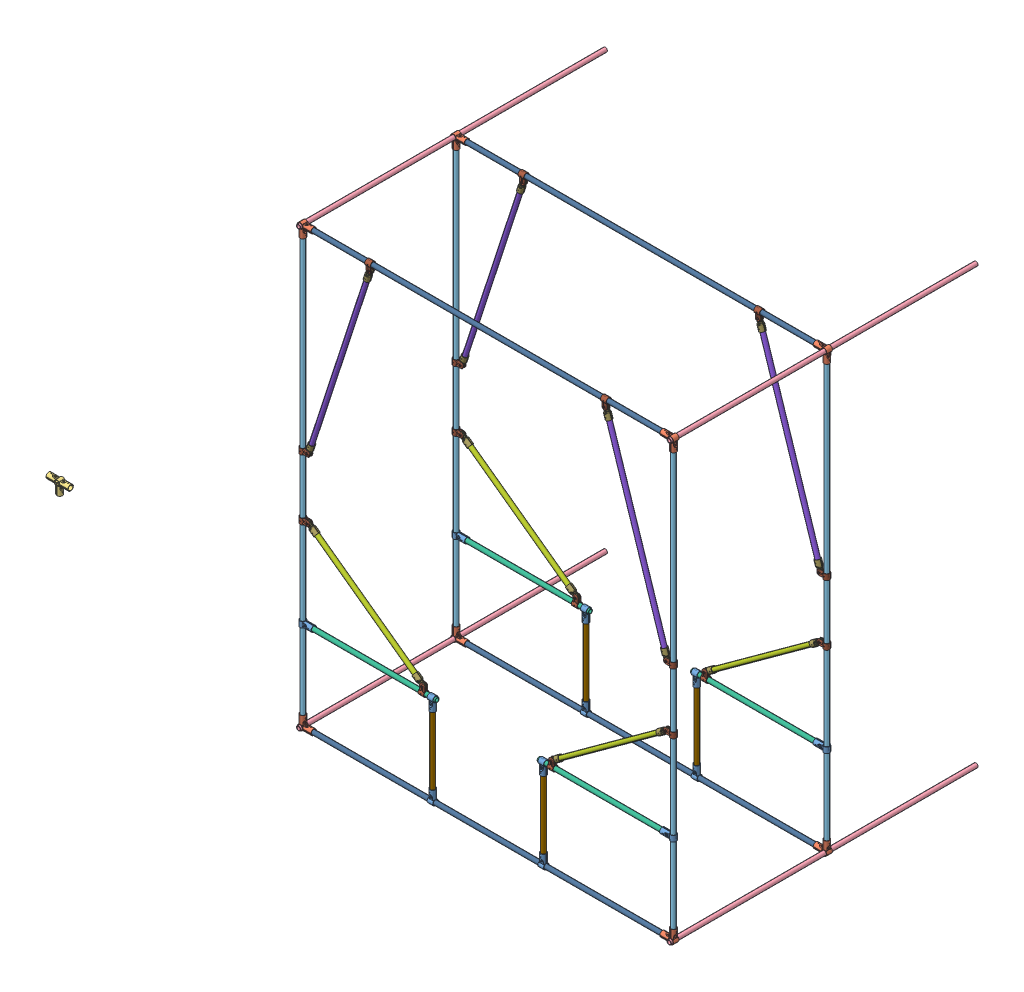
SolidWorks assembly SteelTubeAssembly1, configuration Default. Lengths in mm.
Overall size (3684.85 2626.23 1877.32).
97 component instances, 12 part files, 70 mates.
Components (placement in the parent):
- 2534T210_CLAMP-ON FRAMING FITTING-2: 2534T210_CLAMP-ON FRAMING FITTING [2534T21] at (736.6 0 0) x (1 0 0) z (0 0 -1) size (33.53 82.55 34.1)
- 2534T240_CLAMP-ON FRAMING FITTING-1: 2534T240_CLAMP-ON FRAMING FITTING [2534T24] at (2171.7 0 0) x (-1 0 0) z (0 0 1) size (81.85 81.28 33.46)
- 2534T260_CLAMP-ON FRAMING FITTING-1: 2534T260_CLAMP-ON FRAMING FITTING [2534T26] at (-1430.376 594.6399 57.1912) size (130.05 82.36 33.46)
- Depth Bar-1: Depth Bar [Default] at (-38.1 0 -1803.4) x (0 0 1) z (-1 0 0) size (1828.8 25.4 25.4)
- Height-1: Height [Default] at (2171.7 2552.7 0) x (0 -1 0) z (-0.85323 0 -0.521535) size (2514.6 25.4 25.4)
- Horizonal Corner-1: Horizonal Corner [Default] at (0 533.4 0) x (1 0 0) z (0 0.49668 0.867934) size (762 25.4 25.4)
- Lower Mounting Bar-1: Lower Mounting Bar [Default] at (37.4552 1037.0521 0) x (0.809017 -0.587785 0) z (0.370288 0.509658 0.776618) size (762 25.4 25.4)
- Upper Mounting Bar-1: Upper Mounting Bar [Default] at (7.9592 1459.4984 0) x (0.309017 0.951057 0) z (0.948348 -0.308137 -0.075413) size (1117.6 25.4 25.4)
- Vertical Corner-1: Vertical Corner [Default] at (736.6 495.3 0) x (0 -1 0) z (-0.989698 0 0.143171) size (457.2 25.4 25.4)
- Width-1: Width [Default] at origin size (2133.6 25.4 25.4)
- 2534T240_CLAMP-ON FRAMING FITTING-2: 2534T240_CLAMP-ON FRAMING FITTING [2534T24] at (2171.7 2590.8 0) x (-1 0 0) z (0 0 -1) size (81.85 81.28 33.46)
- 2534T240_CLAMP-ON FRAMING FITTING-5: 2534T240_CLAMP-ON FRAMING FITTING [2534T24] at (-38.1 0 0) x (1 0 0) z (0 0 -1) size (81.85 81.28 33.46)
- Height-3: Height [Default] at (-38.1 2552.7 0) x (0 -1 0) z (-0.845396 0 -0.534139) size (2514.6 25.4 25.4)
- 2534T240_CLAMP-ON FRAMING FITTING-6: 2534T240_CLAMP-ON FRAMING FITTING [2534T24] at (-38.1 2590.8 0) size (81.85 81.28 33.46)
- Width-3: Width [Default] at (0 2590.8 0) x (1 0 0) z (0 0.262637 0.964895) size (2133.6 25.4 25.4)
- 2534T210_CLAMP-ON FRAMING FITTING-3: 2534T210_CLAMP-ON FRAMING FITTING [2534T21] at (736.6 533.4 0) size (33.53 82.55 34.1)
- 2534T210_CLAMP-ON FRAMING FITTING-5: 2534T210_CLAMP-ON FRAMING FITTING [2534T21] at (-38.1 533.4 0) x (0 -1 0) z (0 0 -1) size (33.53 82.55 34.1)
- 2534T210_CLAMP-ON FRAMING FITTING-10: 2534T210_CLAMP-ON FRAMING FITTING [2534T21] at (1397 0 0) x (1 0 0) z (0 0 -1) size (33.53 82.55 34.1)
- 2534T210_CLAMP-ON FRAMING FITTING-11: 2534T210_CLAMP-ON FRAMING FITTING [2534T21] at (1397 533.4 0) x (-1 0 0) z (0 0 -1) size (33.53 82.55 34.1)
- Vertical Corner-3: Vertical Corner [Default] at (1397 495.3 0) x (0 -1 0) z (-0.962184 0 -0.272399) size (457.2 25.4 25.4)
- Horizonal Corner-3: Horizonal Corner [Default] at (1371.6 533.4 0) x (1 0 0) z (0 -0.195703 0.980663) size (762 25.4 25.4)
- 2534T210_CLAMP-ON FRAMING FITTING-12: 2534T210_CLAMP-ON FRAMING FITTING [2534T21] at (2171.7 533.4 0) x (0 -1 0) z (0 0 1) size (33.53 82.55 34.1)
- Adjustable_18deg-1: Adjustable_18deg [Default] at (32.4607 1398.2418 -8.9201) size (87.05 82.3 33.53)
  - Adjustable Connector Part 1-1: Adjustable Connector Part 1 [2534T33] at (-70.5607 28.1617 8.9201) size (68.33 33.53 33.53)
  - Adjustable Connector Part 2-1: Adjustable Connector Part 2 [2534T33] at (-46.1648 -5.4163 8.9201) x (0.309017 0.951057 0) z (0 0 1) size (75.66 33.46 33.53)
- Adjustable_36deg-1: Adjustable_36deg [Default] at (710.24 603.9607 -8.9201) x (0 1 0) z (0 0 1) size (101.88 80.88 33.53)
  - Adjustable Connector Part 1-1: Adjustable Connector Part 1 [2534T33] at (-70.5607 28.1617 8.9201) size (68.33 33.53 33.53)
  - Adjustable Connector Part 2-1: Adjustable Connector Part 2 [2534T33] at (-56.007 -0.4015 8.9201) x (0.587785 0.809017 0) z (0 0 1) size (75.66 33.46 33.53)
- Adjustable_54deg-1: Adjustable_54deg [Default] at (32.4607 1094.4566 8.9201) x (1 0 0) z (0 0 -1) size (111.84 71.54 33.53)
  - Adjustable Connector Part 1-1: Adjustable Connector Part 1 [2534T33] at (-70.5607 28.1617 8.9201) size (68.33 33.53 33.53)
  - Adjustable Connector Part 2-1: Adjustable Connector Part 2 [2534T33] at (-63.8178 7.4093 8.9201) x (0.809017 0.587785 0) z (0 0 1) size (75.66 33.46 33.53)
- Adjustable_72deg-1: Adjustable_72deg [Default] at (392.2314 2520.2393 8.9201) x (0 -1 0) z (0 0 -1) size (115.94 55.2 33.53)
  - Adjustable Connector Part 1-1: Adjustable Connector Part 1 [2534T33] at (-70.5607 28.1617 8.9201) size (68.33 33.53 33.53)
  - Adjustable Connector Part 2-1: Adjustable Connector Part 2 [2534T33] at (-68.8327 17.2515 8.9201) x (0.951057 0.309017 0) z (0 0 1) size (75.66 33.46 33.53)
- Adjustable_72deg-2: Adjustable_72deg [Default] at (1741.3686 2520.2393 -8.9201) x (0 -1 0) z (0 0 1) size (115.94 55.2 33.53)
  - Adjustable Connector Part 1-1: Adjustable Connector Part 1 [2534T33] at (-70.5607 28.1617 8.9201) size (68.33 33.53 33.53)
  - Adjustable Connector Part 2-1: Adjustable Connector Part 2 [2534T33] at (-68.8327 17.2515 8.9201) x (0.951057 0.309017 0) z (0 0 1) size (75.66 33.46 33.53)
- Upper Mounting Bar-2: Upper Mounting Bar [Default] at (2125.6408 1459.4984 0) x (-0.309017 0.951057 0) z (0.948348 0.308137 0.075413) size (1117.6 25.4 25.4)
- Adjustable_18deg-2: Adjustable_18deg [Default] at (2101.1393 1398.2418 8.9201) x (-1 0 0) z (0 0 -1) size (87.05 82.3 33.53)
  - Adjustable Connector Part 1-1: Adjustable Connector Part 1 [2534T33] at (-70.5607 28.1617 8.9201) size (68.33 33.53 33.53)
  - Adjustable Connector Part 2-1: Adjustable Connector Part 2 [2534T33] at (-46.1648 -5.4163 8.9201) x (0.309017 0.951057 0) z (0 0 1) size (75.66 33.46 33.53)
- Adjustable_36deg-2: Adjustable_36deg [Default] at (1423.36 603.9607 8.9201) x (0 1 0) z (0 0 -1) size (101.88 80.88 33.53)
  - Adjustable Connector Part 1-1: Adjustable Connector Part 1 [2534T33] at (-70.5607 28.1617 8.9201) size (68.33 33.53 33.53)
  - Adjustable Connector Part 2-1: Adjustable Connector Part 2 [2534T33] at (-56.007 -0.4015 8.9201) x (0.587785 0.809017 0) z (0 0 1) size (75.66 33.46 33.53)
- Lower Mounting Bar-2: Lower Mounting Bar [Default] at (2096.1448 1037.0521 0) x (-0.809017 -0.587785 0) z (0.370288 -0.509658 -0.776618) size (762 25.4 25.4)
- Adjustable_54deg-2: Adjustable_54deg [Default] at (2101.1393 1094.4566 -8.9201) x (-1 0 0) z (0 0 1) size (111.84 71.54 33.53)
  - Adjustable Connector Part 1-1: Adjustable Connector Part 1 [2534T33] at (-70.5607 28.1617 8.9201) size (68.33 33.53 33.53)
  - Adjustable Connector Part 2-1: Adjustable Connector Part 2 [2534T33] at (-63.8178 7.4093 8.9201) x (0.809017 0.587785 0) z (0 0 1) size (75.66 33.46 33.53)
- Width-4: Width [Default] at (0 2590.8 -914.4) x (1 0 0) z (0 -0.262637 0.964895) size (2133.6 25.4 25.4)
- Height-4: Height [Default] at (-38.1 2552.7 -914.4) x (0 -1 0) z (0.845396 0 -0.534139) size (2514.6 25.4 25.4)
- 2534T240_CLAMP-ON FRAMING FITTING-7: 2534T240_CLAMP-ON FRAMING FITTING [2534T24] at (-38.1 2590.8 -914.4) size (81.85 81.28 33.46)
- Upper Mounting Bar-3: Upper Mounting Bar [Default] at (7.9592 1459.4984 -914.4) x (0.309017 0.951057 0) z (-0.948348 0.308137 -0.075413) size (1117.6 25.4 25.4)
- Adjustable_72deg-3: Adjustable_72deg [Default] at (392.2314 2520.2393 -905.4799) x (0 -1 0) z (0 0 -1) size (115.94 55.2 33.53)
  - Adjustable Connector Part 1-1: Adjustable Connector Part 1 [2534T33] at (-70.5607 28.1617 8.9201) size (68.33 33.53 33.53)
  - Adjustable Connector Part 2-1: Adjustable Connector Part 2 [2534T33] at (-68.8327 17.2515 8.9201) x (0.951057 0.309017 0) z (0 0 1) size (75.66 33.46 33.53)
- Adjustable_54deg-3: Adjustable_54deg [Default] at (32.4607 1094.4566 -905.4799) x (1 0 0) z (0 0 -1) size (111.84 71.54 33.53)
  - Adjustable Connector Part 1-1: Adjustable Connector Part 1 [2534T33] at (-70.5607 28.1617 8.9201) size (68.33 33.53 33.53)
  - Adjustable Connector Part 2-1: Adjustable Connector Part 2 [2534T33] at (-63.8178 7.4093 8.9201) x (0.809017 0.587785 0) z (0 0 1) size (75.66 33.46 33.53)
- Adjustable_18deg-3: Adjustable_18deg [Default] at (32.4607 1398.2418 -923.3201) size (87.05 82.3 33.53)
  - Adjustable Connector Part 1-1: Adjustable Connector Part 1 [2534T33] at (-70.5607 28.1617 8.9201) size (68.33 33.53 33.53)
  - Adjustable Connector Part 2-1: Adjustable Connector Part 2 [2534T33] at (-46.1648 -5.4163 8.9201) x (0.309017 0.951057 0) z (0 0 1) size (75.66 33.46 33.53)
- Lower Mounting Bar-3: Lower Mounting Bar [Default] at (37.4552 1037.0521 -914.4) x (0.809017 -0.587785 0) z (-0.370288 -0.509658 0.776618) size (762 25.4 25.4)
- Horizonal Corner-4: Horizonal Corner [Default] at (0 533.4 -914.4) x (1 0 0) z (0 -0.49668 0.867934) size (762 25.4 25.4)
- 2534T210_CLAMP-ON FRAMING FITTING-13: 2534T210_CLAMP-ON FRAMING FITTING [2534T21] at (-38.1 533.4 -914.4) x (0 1 0) z (0 0 1) size (33.53 82.55 34.1)
- Adjustable_36deg-3: Adjustable_36deg [Default] at (710.24 603.9607 -923.3201) x (0 1 0) z (0 0 1) size (101.88 80.88 33.53)
  - Adjustable Connector Part 1-1: Adjustable Connector Part 1 [2534T33] at (-70.5607 28.1617 8.9201) size (68.33 33.53 33.53)
  - Adjustable Connector Part 2-1: Adjustable Connector Part 2 [2534T33] at (-56.007 -0.4015 8.9201) x (0.587785 0.809017 0) z (0 0 1) size (75.66 33.46 33.53)
- Vertical Corner-4: Vertical Corner [Default] at (736.6 495.3 -914.4) x (0 -1 0) z (0.989698 0 0.143171) size (457.2 25.4 25.4)
- 2534T210_CLAMP-ON FRAMING FITTING-14: 2534T210_CLAMP-ON FRAMING FITTING [2534T21] at (736.6 533.4 -914.4) x (-1 0 0) z (0 0 -1) size (33.53 82.55 34.1)
- Width-5: Width [Default] at (0 0 -914.4) size (2133.6 25.4 25.4)
- 2534T240_CLAMP-ON FRAMING FITTING-8: 2534T240_CLAMP-ON FRAMING FITTING [2534T24] at (-38.1 0 -914.4) x (1 0 0) z (0 0 -1) size (81.85 81.28 33.46)
- Adjustable_54deg-4: Adjustable_54deg [Default] at (2101.1393 1094.4566 -923.3201) x (-1 0 0) z (0 0 1) size (111.84 71.54 33.53)
  - Adjustable Connector Part 1-1: Adjustable Connector Part 1 [2534T33] at (-70.5607 28.1617 8.9201) size (68.33 33.53 33.53)
  - Adjustable Connector Part 2-1: Adjustable Connector Part 2 [2534T33] at (-63.8178 7.4093 8.9201) x (0.809017 0.587785 0) z (0 0 1) size (75.66 33.46 33.53)
- Lower Mounting Bar-4: Lower Mounting Bar [Default] at (2096.1448 1037.0521 -914.4) x (-0.809017 -0.587785 0) z (-0.370288 0.509658 -0.776618) size (762 25.4 25.4)
- Upper Mounting Bar-4: Upper Mounting Bar [Default] at (2125.6408 1459.4984 -914.4) x (-0.309017 0.951057 0) z (-0.948348 -0.308137 0.075413) size (1117.6 25.4 25.4)
- Adjustable_36deg-4: Adjustable_36deg [Default] at (1423.36 603.9607 -905.4799) x (0 1 0) z (0 0 -1) size (101.88 80.88 33.53)
  - Adjustable Connector Part 1-1: Adjustable Connector Part 1 [2534T33] at (-70.5607 28.1617 8.9201) size (68.33 33.53 33.53)
  - Adjustable Connector Part 2-1: Adjustable Connector Part 2 [2534T33] at (-56.007 -0.4015 8.9201) x (0.587785 0.809017 0) z (0 0 1) size (75.66 33.46 33.53)
- Adjustable_18deg-4: Adjustable_18deg [Default] at (2101.1393 1398.2418 -905.4799) x (-1 0 0) z (0 0 -1) size (87.05 82.3 33.53)
  - Adjustable Connector Part 1-1: Adjustable Connector Part 1 [2534T33] at (-70.5607 28.1617 8.9201) size (68.33 33.53 33.53)
  - Adjustable Connector Part 2-1: Adjustable Connector Part 2 [2534T33] at (-46.1648 -5.4163 8.9201) x (0.309017 0.951057 0) z (0 0 1) size (75.66 33.46 33.53)
- Adjustable_72deg-4: Adjustable_72deg [Default] at (1741.3686 2520.2393 -923.3201) x (0 -1 0) z (0 0 1) size (115.94 55.2 33.53)
  - Adjustable Connector Part 1-1: Adjustable Connector Part 1 [2534T33] at (-70.5607 28.1617 8.9201) size (68.33 33.53 33.53)
  - Adjustable Connector Part 2-1: Adjustable Connector Part 2 [2534T33] at (-68.8327 17.2515 8.9201) x (0.951057 0.309017 0) z (0 0 1) size (75.66 33.46 33.53)
- 2534T210_CLAMP-ON FRAMING FITTING-15: 2534T210_CLAMP-ON FRAMING FITTING [2534T21] at (1397 0 -913.8268) x (1 0 0) z (0 0 -1) size (33.53 82.55 34.1)
- 2534T210_CLAMP-ON FRAMING FITTING-16: 2534T210_CLAMP-ON FRAMING FITTING [2534T21] at (2171.7 533.4 -914.4) x (0 1 0) z (0 0 -1) size (33.53 82.55 34.1)
- Horizonal Corner-5: Horizonal Corner [Default] at (1371.6 533.4 -914.4) x (1 0 0) z (0 0.195703 0.980663) size (762 25.4 25.4)
- Vertical Corner-5: Vertical Corner [Default] at (1397 495.3 -914.4) x (0 -1 0) z (0.962184 0 -0.272399) size (457.2 25.4 25.4)
- 2534T210_CLAMP-ON FRAMING FITTING-17: 2534T210_CLAMP-ON FRAMING FITTING [2534T21] at (1397 533.4 -913.8268) x (-1 0 0) z (0 0 -1) size (33.53 82.55 34.1)
- 2534T240_CLAMP-ON FRAMING FITTING-9: 2534T240_CLAMP-ON FRAMING FITTING [2534T24] at (2171.7 2590.8 -914.4) x (-1 0 0) z (0 0 -1) size (81.85 81.28 33.46)
- 2534T210_CLAMP-ON FRAMING FITTING-18: 2534T210_CLAMP-ON FRAMING FITTING [2534T21] at (736.6 0 -913.8268) x (1 0 0) z (0 0 -1) size (33.53 82.55 34.1)
- 2534T240_CLAMP-ON FRAMING FITTING-10: 2534T240_CLAMP-ON FRAMING FITTING [2534T24] at (2171.7 0 -914.4) x (-1 0 0) z (0 0 1) size (81.85 81.28 33.46)
- Height-5: Height [Default] at (2171.7 2552.7 -914.4) x (0 -1 0) z (0.85323 0 -0.521535) size (2514.6 25.4 25.4)
- Depth Bar-2: Depth Bar [Default] at (2171.7 0 25.4) x (0 0 -1) z (0.840422 0.541932 0) size (1828.8 25.4 25.4)
- Depth Bar-3: Depth Bar [Default] at (-38.1 2590.8 25.4) x (0 0 -1) z (-0.633686 -0.77359 0) size (1828.8 25.4 25.4)
- Depth Bar-4: Depth Bar [Default] at (2171.7 2590.8 -1803.4) x (0 0 1) z (-0.806438 -0.591319 0) size (1828.8 25.4 25.4)
Mates (geometry in assembly coordinates):
- Coincident1: coordinate: point of Width-1; point of assembly
- Concentric1: concentric anti-aligned: cylinder of 2534T240_CLAMP-ON FRAMING FITTING-1 through (2107.184 0 0) axis (1 0 0) radius 13.97; cylinder of Width-1 through (2133.6 0 0) axis (-1 0 0) radius 12.7
- Distance1: distance = 38.1 mm: point of 2534T240_CLAMP-ON FRAMING FITTING-1; plane of Width-1 through (2133.6 0 0) normal (1 0 0)
- Coincident2: coincident aligned: plane of Width-1 through (0 0 0) normal (0 0 1); plane of assembly through (0 0 0) normal (0 0 1)
- Parallel1: parallel aligned: plane of 2534T240_CLAMP-ON FRAMING FITTING-1 through (2171.7 64.516 0) normal (0 1 0); plane of assembly through (0 0 0) normal (0 1 0)
- Concentric2: concentric anti-aligned: cylinder of 2534T240_CLAMP-ON FRAMING FITTING-1 through (2171.7 64.516 0) axis (0 -1 0) radius 13.97; cylinder of Height-1 through (2171.7 38.1 0) axis (0 1 0) radius 12.7
- Distance2: distance = 38.1 mm anti-aligned: plane of Height-1 through (2171.7 38.1 0) normal (0 -1 0); plane of Width-1 through (0 0 0) normal (0 1 0)
- Concentric3: concentric aligned: cylinder of Height-1 through (2171.7 38.1 0) axis (0 1 0) radius 12.7; cylinder of 2534T240_CLAMP-ON FRAMING FITTING-2 through (2171.7 2526.284 0) axis (0 1 0) radius 13.97
- Distance3: distance = 38.1 mm: plane of Height-1 through (2171.7 2552.7 0) normal (0 1 0); point of 2534T240_CLAMP-ON FRAMING FITTING-2
- Parallel2: parallel aligned: plane of 2534T240_CLAMP-ON FRAMING FITTING-2 through (2171.7 2590.8 16.73) normal (0 0 1); plane of assembly through (0 0 0) normal (0 0 1)
- Concentric13: concentric aligned: cylinder of Width-1 through (2133.6 0 0) axis (-1 0 0) radius 12.7; cylinder of 2534T240_CLAMP-ON FRAMING FITTING-5 through (26.416 0 0) axis (-1 0 0) radius 13.97
- Distance9: distance = 38.1 mm: plane of Width-1 through (0 0 0) normal (-1 0 0); point of 2534T240_CLAMP-ON FRAMING FITTING-5
- Parallel5: parallel aligned: plane of 2534T240_CLAMP-ON FRAMING FITTING-1 through (2171.7 64.516 0) normal (0 1 0); plane of 2534T240_CLAMP-ON FRAMING FITTING-5 through (-38.1 64.516 0) normal (0 1 0)
- Concentric14: concentric anti-aligned: cylinder of 2534T240_CLAMP-ON FRAMING FITTING-5 through (-38.1 64.516 0) axis (0 -1 0) radius 13.97; cylinder of Height-3 through (-38.1 38.1 0) axis (0 1 0) radius 12.7
- Distance10: distance = 38.1 mm: plane of Height-3 through (-38.1 38.1 0) normal (0 -1 0); point of 2534T240_CLAMP-ON FRAMING FITTING-5
- Concentric15: concentric aligned: cylinder of Height-3 through (-38.1 38.1 0) axis (0 1 0) radius 12.7; cylinder of 2534T240_CLAMP-ON FRAMING FITTING-6 through (-38.1 2526.284 0) axis (0 1 0) radius 13.97
- Distance11: distance = 38.1 mm: plane of Height-3 through (-38.1 2552.7 0) normal (0 1 0); point of 2534T240_CLAMP-ON FRAMING FITTING-6
- Parallel6: parallel aligned: plane of Height-1 through (2171.7 2552.7 0) normal (0 1 0); plane of Height-3 through (-38.1 2552.7 0) normal (0 1 0)
- Concentric16: concentric anti-aligned: cylinder of 2534T240_CLAMP-ON FRAMING FITTING-2 through (2107.184 2590.8 0) axis (1 0 0) radius 13.97; cylinder of Width-3 through (2133.6 2590.8 0) axis (-1 0 0) radius 12.7
- Distance12: distance = 38.1 mm: point of 2534T240_CLAMP-ON FRAMING FITTING-2; plane of Width-3 through (2133.6 2590.8 0) normal (1 0 0)
- Parallel8: parallel anti-aligned: plane of 2534T240_CLAMP-ON FRAMING FITTING-2 through (2107.184 2590.8 0) normal (-1 0 0); plane of 2534T240_CLAMP-ON FRAMING FITTING-6 through (26.416 2590.8 0) normal (1 0 0)
- Concentric19: concentric aligned: cylinder of 2534T210_CLAMP-ON FRAMING FITTING-2 through (753.364 0 0) axis (-1 0 0) radius 13.97; cylinder of Width-1 through (2133.6 0 0) axis (-1 0 0) radius 12.7
- Parallel9: parallel aligned: plane of 2534T210_CLAMP-ON FRAMING FITTING-2 through (736.6 65.786 0) normal (0 1 0); plane of 2534T240_CLAMP-ON FRAMING FITTING-5 through (-38.1 64.516 0) normal (0 1 0)
- Concentric20: concentric anti-aligned: cylinder of 2534T210_CLAMP-ON FRAMING FITTING-2 through (736.6 65.786 0) axis (0 -1 0) radius 13.97; cylinder of Vertical Corner-1 through (736.6 38.1 0) axis (0 1 0) radius 12.7
- Distance13: distance = 38.1 mm: point of 2534T210_CLAMP-ON FRAMING FITTING-2; plane of Vertical Corner-1 through (736.6 38.1 0) normal (0 -1 0)
- Concentric24: concentric aligned: cylinder of Vertical Corner-1 through (736.6 38.1 0) axis (0 1 0) radius 12.7; cylinder of 2534T210_CLAMP-ON FRAMING FITTING-3 through (736.6 467.614 0) axis (0 1 0) radius 13.97
- Distance14: distance = 38.1 mm: point of 2534T210_CLAMP-ON FRAMING FITTING-3; plane of Vertical Corner-1 through (736.6 495.3 0) normal (0 1 0)
- Concentric25: concentric anti-aligned: cylinder of Height-3 through (-38.1 38.1 0) axis (0 1 0) radius 12.7; cylinder of 2534T210_CLAMP-ON FRAMING FITTING-5 through (-38.1 550.164 0) axis (0 -1 0) radius 13.97
- Parallel10: parallel aligned: plane of 2534T240_CLAMP-ON FRAMING FITTING-5 through (26.416 0 0) normal (1 0 0); plane of 2534T210_CLAMP-ON FRAMING FITTING-5 through (27.686 533.4 0) normal (1 0 0)
- Parallel11: parallel anti-aligned: plane of 2534T210_CLAMP-ON FRAMING FITTING-3 through (719.836 533.4 0) normal (-1 0 0); plane of 2534T210_CLAMP-ON FRAMING FITTING-5 through (27.686 533.4 0) normal (1 0 0)
- Concentric26: concentric aligned: cylinder of Horizonal Corner-1 through (762 533.4 0) axis (-1 0 0) radius 12.7; cylinder of 2534T210_CLAMP-ON FRAMING FITTING-3 through (753.364 533.4 0) axis (-1 0 0) radius 13.97
- Distance15: distance = 25.4 mm: point of 2534T210_CLAMP-ON FRAMING FITTING-3; plane of Horizonal Corner-1 through (762 533.4 0) normal (1 0 0)
- Distance16: distance = 38.1 mm: plane of Horizonal Corner-1 through (0 533.4 0) normal (-1 0 0); point of 2534T210_CLAMP-ON FRAMING FITTING-5
- Concentric27: concentric aligned: cylinder of Horizonal Corner-1 through (762 533.4 0) axis (-1 0 0) radius 12.7; cylinder of 2534T210_CLAMP-ON FRAMING FITTING-5 through (27.686 533.4 0) axis (-1 0 0) radius 13.97
- Concentric28: concentric aligned: cylinder of ? through (569.8292 2128.6091 5503.5233) axis (0 1 0) radius 12.7; cylinder of ? through (569.8292 2558.1231 5503.5233) axis (0 1 0) radius 13.97
- Distance17: distance = 25.4 mm: point of ?; plane of ? through (595.2292 2623.9091 5503.5233) normal (1 0 0)
- Distance19: distance = 38.1 mm: point of ?; plane of ? through (569.8292 2585.8091 5503.5233) normal (0 1 0)
- Concentric30: concentric aligned: cylinder of ? through (595.2292 2623.9091 5503.5233) axis (-1 0 0) radius 12.7; cylinder of ? through (586.5932 2623.9091 5503.5233) axis (-1 0 0) radius 13.97
- Concentric31: concentric anti-aligned: cylinder of Width-1 through (2133.6 0 0) axis (-1 0 0) radius 12.7; cylinder of 2534T210_CLAMP-ON FRAMING FITTING-10 through (1380.236 0 0) axis (1 0 0) radius 13.97
- Concentric32: concentric anti-aligned: cylinder of 2534T210_CLAMP-ON FRAMING FITTING-10 through (1397 65.786 0) axis (0 -1 0) radius 13.97; cylinder of Vertical Corner-3 through (1397 38.1 0) axis (0 1 0) radius 12.7
- Distance20: distance = 38.1 mm: plane of Vertical Corner-3 through (1397 38.1 0) normal (0 -1 0); point of 2534T210_CLAMP-ON FRAMING FITTING-10
- Concentric33: concentric aligned: cylinder of 2534T210_CLAMP-ON FRAMING FITTING-11 through (1397 467.614 0) axis (0 1 0) radius 13.97; cylinder of Vertical Corner-3 through (1397 38.1 0) axis (0 1 0) radius 12.7
- Parallel12: parallel aligned: plane of 2534T240_CLAMP-ON FRAMING FITTING-1 through (2171.7 64.516 0) normal (0 1 0); plane of Vertical Corner-3 through (1397 495.3 0) normal (0 1 0)
- Distance21: distance = 38.1 mm: point of 2534T210_CLAMP-ON FRAMING FITTING-11; plane of Vertical Corner-3 through (1397 495.3 0) normal (0 1 0)
- Parallel13: parallel anti-aligned: plane of 2534T210_CLAMP-ON FRAMING FITTING-3 through (753.364 533.4 0) normal (1 0 0); plane of 2534T210_CLAMP-ON FRAMING FITTING-11 through (1380.236 533.4 0) normal (-1 0 0)
- Concentric34: concentric aligned: cylinder of 2534T210_CLAMP-ON FRAMING FITTING-11 through (1413.764 533.4 0) axis (-1 0 0) radius 13.97; cylinder of Horizonal Corner-3 through (2133.6 533.4 0) axis (-1 0 0) radius 12.7
- Distance22: distance = 25.4 mm: point of 2534T210_CLAMP-ON FRAMING FITTING-11; plane of Horizonal Corner-3 through (1371.6 533.4 0) normal (-1 0 0)
- Concentric35: concentric anti-aligned: cylinder of Height-1 through (2171.7 38.1 0) axis (0 1 0) radius 12.7; cylinder of 2534T210_CLAMP-ON FRAMING FITTING-12 through (2171.7 550.164 0) axis (0 -1 0) radius 13.97
- Concentric36: concentric anti-aligned: cylinder of Horizonal Corner-3 through (2133.6 533.4 0) axis (-1 0 0) radius 12.7; cylinder of 2534T210_CLAMP-ON FRAMING FITTING-12 through (2105.914 533.4 0) axis (1 0 0) radius 13.97
- Distance23: distance = 38.1 mm: point of 2534T210_CLAMP-ON FRAMING FITTING-12; plane of Horizonal Corner-3 through (2133.6 533.4 0) normal (1 0 0)
- Concentric37: concentric aligned: cylinder of Height-3 through (-38.1 38.1 0) axis (0 1 0) radius 12.7; cylinder of Adjustable_18deg-1/Adjustable Connector Part 1-1 through (-38.1 1409.6385 0) axis (0 1 0) radius 13.97
- Concentric38: concentric anti-aligned: cylinder of Upper Mounting Bar-1 through (353.3166 2522.3991 0) axis (-0.309017 -0.951057 0) radius 12.7; cylinder of Adjustable_18deg-1/Adjustable Connector Part 2-1 through (4.0347 1447.42 0) axis (0.309017 0.951057 0) radius 13.97
- Concentric39: concentric aligned: cylinder of Width-3 through (2133.6 2590.8 0) axis (-1 0 0) radius 12.7; cylinder of Adjustable_72deg-1/Adjustable Connector Part 1-1 through (380.8347 2590.8 0) axis (-1 0 0) radius 13.97
- Concentric40: concentric aligned: cylinder of Upper Mounting Bar-1 through (353.3166 2522.3991 0) axis (-0.309017 -0.951057 0) radius 12.7; cylinder of Adjustable_72deg-1/Adjustable Connector Part 2-1 through (357.2411 2534.4776 0) axis (-0.309017 -0.951057 0) radius 13.97
- Distance24: distance = 12.7 mm: plane of Upper Mounting Bar-1 through (353.3166 2522.3991 0) normal (0.309017 0.951057 0); line of Adjustable_72deg-1 through (357.2411 2534.4776 -7.4998) axis (0 0 1)
- Distance27: distance = 1083.1165 mm anti-aligned: plane of Adjustable_18deg-1/Adjustable Connector Part 1-1 through (-38.1 1443.1675 0) normal (0 1 0); plane of 2534T240_CLAMP-ON FRAMING FITTING-6 through (-38.1 2526.284 0) normal (0 -1 0)
- Concentric41: concentric aligned: cylinder of Horizonal Corner-1 through (762 533.4 0) axis (-1 0 0) radius 12.7; cylinder of Adjustable_36deg-1/Adjustable Connector Part 1-1 through (698.8434 533.4 0) axis (-1 0 0) radius 13.97
- Concentric42: concentric anti-aligned: cylinder of Height-3 through (-38.1 38.1 0) axis (0 1 0) radius 12.7; cylinder of Adjustable_54deg-1/Adjustable Connector Part 1-1 through (-38.1 1083.0599 0) axis (0 -1 0) radius 13.97
- Concentric43: concentric anti-aligned: cylinder of Lower Mounting Bar-1 through (653.9262 589.1598 0) axis (-0.809017 0.587785 0) radius 12.7; cylinder of Adjustable_54deg-1/Adjustable Connector Part 2-1 through (15.0837 1053.306 0) axis (0.809017 -0.587785 0) radius 13.97
- Concentric44: concentric aligned: cylinder of Lower Mounting Bar-1 through (653.9262 589.1598 0) axis (-0.809017 0.587785 0) radius 12.7; cylinder of Adjustable_36deg-1/Adjustable Connector Part 2-1 through (664.2007 581.6949 0) axis (-0.809017 0.587785 0) radius 13.97
- Distance28: distance = 12.7 mm: plane of Lower Mounting Bar-1 through (653.9262 589.1598 0) normal (0.809017 -0.587785 0); line of Adjustable_36deg-1 through (664.2007 581.6949 7.4998) axis (0 0 -1)
- Distance30: distance = 499.3669 mm anti-aligned: plane of 2534T210_CLAMP-ON FRAMING FITTING-5 through (-38.1 550.164 0) normal (0 1 0); plane of Adjustable_54deg-1/Adjustable Connector Part 1-1 through (-38.1 1049.5309 0) normal (0 -1 0)
- Concentric45: concentric: cylinder of Depth Bar-1 through (-38.1 0 25.4) axis (0 0 -1) radius 12.7; cylinder of 2534T240_CLAMP-ON FRAMING FITTING-5 through (-38.1 0 -16.731) axis (0 0 1) radius 13.97
- Distance31: distance = 25.4 mm: plane of Depth Bar-1 through (-38.1 0 25.4) normal (0 0 1); point of 2534T240_CLAMP-ON FRAMING FITTING-5
- Concentric46: concentric: cylinder of 2534T240_CLAMP-ON FRAMING FITTING-2 through (2171.7 2590.8 -16.731) axis (0 0 1) radius 13.97; cylinder of Depth Bar-4 through (2171.7 2590.8 25.4) axis (0 0 -1) radius 12.7
- Concentric47: concentric: cylinder of 2534T240_CLAMP-ON FRAMING FITTING-1 through (2171.7 0 16.731) axis (0 0 -1) radius 13.97; cylinder of Depth Bar-2 through (2171.7 0 -1705.567) axis (0 0 1) radius 12.7
- Concentric48: concentric: cylinder of 2534T240_CLAMP-ON FRAMING FITTING-6 through (-38.1 2590.8 16.731) axis (0 0 -1) radius 13.97; cylinder of Depth Bar-3 through (-38.1 2590.8 -1803.4) axis (0 0 1) radius 12.7
- Distance32: distance = 25.4 mm: plane of Depth Bar-3 through (-38.1 2590.8 25.4) normal (0 0 1); point of 2534T240_CLAMP-ON FRAMING FITTING-6
- Distance33: distance = 25.4 mm: plane of Depth Bar-4 through (2171.7 2590.8 25.4) normal (0 0 1); point of 2534T240_CLAMP-ON FRAMING FITTING-2
- Distance34: distance = 25.4 mm: plane of Depth Bar-2 through (2171.7 0 25.4) normal (0 0 1); point of 2534T240_CLAMP-ON FRAMING FITTING-1
